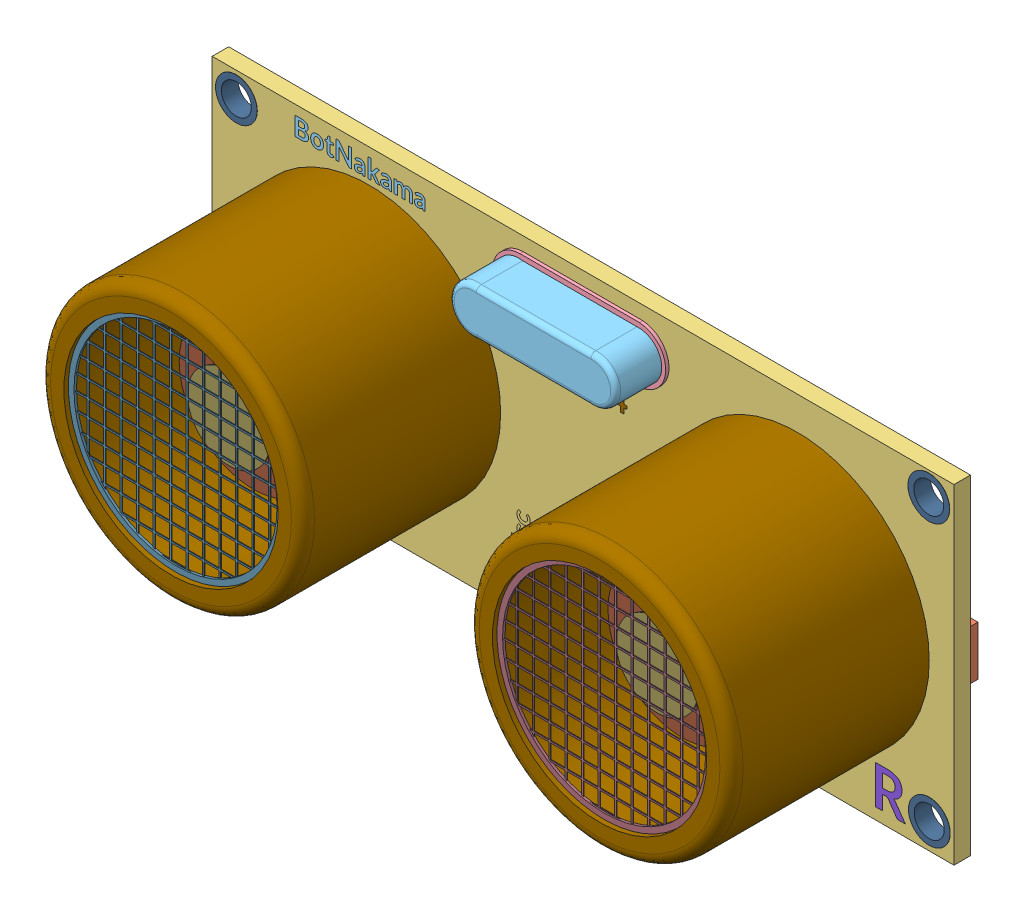
SolidWorks assembly HC-04HC-04, configuration Default. Lengths in mm.
Overall size (45 25.57 17.46).
61 component instances, 60 part files, 0 mates.
Components (placement in the parent):
- HC-04HC-04.stp-1: HC-04HC-04.stp [Default] at origin size (45 25.57 17.46)
  - HC-04Array.stp-1: HC-04Array.stp [Default] at origin size (10.16 2.54 2.54)
  - HC-04Array001.stp-1: HC-04Array001.stp [Default] at (0 0 1) size (8.32 7.52 6.46)
  - HC-04Placa.stp-1: HC-04Placa.stp [Default] at origin size (45 20 1)
  - HC-04Pad003.stp-1: HC-04Pad003.stp [Default] at (0 0 1) size (10.52 3.38 0.2)
  - HC-04Fillet.stp-1: HC-04Fillet.stp [Default] at (0 0 1) size (10.1 2.84 3)
  - HC-04Array002.stp-1: HC-04Array002.stp [Default] at origin size (9.62 2 1)
  - HC-04Array003.stp-1: HC-04Array003.stp [Default] at (0 0 1) size (28 12 0.8)
  - HC-04Fusion.stp-1: HC-04Fusion.stp [Default] at origin size (6 2 1)
  - HC-04Fillet001.stp-1: HC-04Fillet001.stp [Default] at (0 0 1) size (42 16 12)
  - HC-04Pad005.stp-1: HC-04Pad005.stp [Default] at (0 0 1) size (39.16 13 0.2)
  - HC-04Pad006.stp-1: HC-04Pad006.stp [Default] at (0 0 1) size (35.01 9.04 7)
  - HC-04Fusion001.stp-1: HC-04Fusion001.stp [Default] at (0 0 8) size (31 5 1.5)
  - HC-04Clone_of_Fusion002.stp-1: HC-04Clone_of_Fusion002.stp [Default] at (47.2 -5.5 12.6) size (13 13 0.15)
  - HC-04Clone_of_Fusion003.stp-1: HC-04Clone_of_Fusion003.stp [Default] at (21.2 -5.5 12.6) size (13 13 0.15)
  - HC-04Array005.stp-1: HC-04Array005.stp [Default] at origin size (9.62 2 1)
  - HC-04Array002002.stp-1: HC-04Array002002.stp [Default] at (-5.9 0.1 0.15) size (6.57 1.4 0.56)
  - HC-04Clone_of_Array002002.stp-1: HC-04Clone_of_Array002002.stp [Default] at (-23.9 0.1 0.15) size (6.57 1.4 0.56)
  - HC-04Array002003.stp-1: HC-04Array002003.stp [Default] at (-6.05 0 0.15) size (6.57 1.4 0.56)
  - HC-04Clone_of_Array002003.stp-1: HC-04Clone_of_Array002003.stp [Default] at (-24.05 0 0.15) size (6.57 1.4 0.56)
  - HC-04Integrados.stp-1: HC-04Integrados.stp [Default] at origin size (42.14 9 1)
  - HC-04ShapeString.stp-1: HC-04ShapeString.stp [Default] at (-3.2 -7 1.01) x (0 1 0) z (0 0 1) size (2.53 1.13 0.01)
  - HC-04ShapeString001.stp-1: HC-04ShapeString001.stp [Default] at (-0.6 -7 1.01) x (0 1 0) z (0 0 1) size (2.66 1.45 0.01)
  - HC-04ShapeString002.stp-1: HC-04ShapeString002.stp [Default] at (1.9 -7 1.01) x (0 1 0) z (0 0 1) size (3.21 1.16 0.01)
  - HC-04ShapeString003.stp-1: HC-04ShapeString003.stp [Default] at (4.5 -7 1.01) x (0 1 0) z (0 0 1) size (2.71 1.16 0.01)
  - HC-04ShapeString004.stp-1: HC-04ShapeString004.stp [Default] at (-19.5 -9.3 1.01) size (1.84 2.34 0.01)
  - HC-04ShapeString005.stp-1: HC-04ShapeString005.stp [Default] at (17.5 -9.3 1.01) size (1.82 2.34 0.01)
  - HC-04ShapeString006.stp-1: HC-04ShapeString006.stp [Default] at (-3 3.7 1.01) size (5.52 1.41 0.01)
  - HC-04Pad008.stp-1: HC-04Pad008.stp [Default] at (0 0 -0.01) size (44.56 19.6 1.02)
  - HC-04Scale004.stp-1: HC-04Scale004.stp [Default] at (-1.9 -21.5 -1.5) x (0 1 0) z (0 0 1) size (0.8 1.77 0.5)
  - HC-04Scale027.stp-1: HC-04Scale027.stp [Default] at (-1.9 -10.2323 -1.5) x (0 1 0) z (0 0 1) size (0.8 1.77 0.5)
  - HC-04Scale028.stp-1: HC-04Scale028.stp [Default] at (8.5984 -21.5 -1.5) x (0 1 0) z (0 0 1) size (0.8 1.77 0.5)
  - HC-04Scale029.stp-1: HC-04Scale029.stp [Default] at (8.5984 -19.5867 -1.5) x (0 1 0) z (0 0 1) size (0.8 1.77 0.5)
  - HC-04Scale030.stp-1: HC-04Scale030.stp [Default] at (8.5984 -17.5982 -1.5) x (0 1 0) z (0 0 1) size (0.8 1.77 0.5)
  - HC-04Scale031.stp-1: HC-04Scale031.stp [Default] at (8.5984 -15.6427 -1.5) x (0 1 0) z (0 0 1) size (0.8 1.77 0.5)
  - HC-04Scale032.stp-1: HC-04Scale032.stp [Default] at (8.5984 -11.6848 -1.5) x (0 1 0) z (0 0 1) size (0.8 1.77 0.5)
  - HC-04Scale033.stp-1: HC-04Scale033.stp [Default] at (-26.74 -2 -1.5) x (0 1 0) z (0 0 1) size (0.8 1.85 0.5)
  - HC-04Scale034.stp-1: HC-04Scale034.stp [Default] at (24.9371 -21.5 -1.5) x (0 1 0) z (0 0 1) size (0.8 1.77 0.5)
  - HC-04Scale035.stp-1: HC-04Scale035.stp [Default] at (24.9691 -19.5867 -1.5) x (0 1 0) z (0 0 1) size (0.8 1.77 0.5)
  - HC-04Scale036.stp-1: HC-04Scale036.stp [Default] at (24.9742 -17.5982 -1.5) x (0 1 0) z (0 0 1) size (0.8 1.77 0.5)
  - HC-04Scale037.stp-1: HC-04Scale037.stp [Default] at (-10.4013 -2 -1.5) x (0 1 0) z (0 0 1) size (0.8 1.85 0.5)
  - HC-04Scale038.stp-1: HC-04Scale038.stp [Default] at (-10.4013 -3.9266 -1.5) x (0 1 0) z (0 0 1) size (0.8 1.85 0.5)
  - HC-04Scale039.stp-1: HC-04Scale039.stp [Default] at (-10.4013 -0.0734 -1.5) x (0 1 0) z (0 0 1) size (0.8 1.85 0.5)
  - HC-04Scale040.stp-1: HC-04Scale040.stp [Default] at (24.9742 -9.855 -1.5) x (0 1 0) z (0 0 1) size (0.8 1.77 0.5)
  - HC-04Scale041.stp-1: HC-04Scale041.stp [Default] at (26.5673 -24.0564 -1.5) x (0 1 0) z (0 0 1) size (0.8 1.77 0.5)
  - HC-04Scale042.stp-1: HC-04Scale042.stp [Default] at (26.5673 -7.3333 -1.5) x (0 1 0) z (0 0 1) size (0.8 1.77 0.5)
  - HC-04Scale043.stp-1: HC-04Scale043.stp [Default] at (30.1435 -7.3333 -1.5) x (0 1 0) z (0 0 1) size (0.8 1.77 0.5)
  - HC-04Scale044.stp-1: HC-04Scale044.stp [Default] at (33.5459 -7.3333 -1.5) x (0 1 0) z (0 0 1) size (0.8 1.77 0.5)
  - HC-04Scale045.stp-1: HC-04Scale045.stp [Default] at (37.7181 -11.1827 -1.5) x (0 1 0) z (0 0 1) size (0.8 1.77 0.5)
  - HC-04Scale046.stp-1: HC-04Scale046.stp [Default] at (37.7181 -20.5932 -1.5) x (0 1 0) z (0 0 1) size (0.8 1.77 0.5)
  - HC-04Scale047.stp-1: HC-04Scale047.stp [Default] at (-3.9042 -12.3288 -1.5) x (0 1 0) z (0 0 1) size (0.8 1.85 0.5)
  - HC-04Scale048.stp-1: HC-04Scale048.stp [Default] at (13.5402 13.2894 -1.5) size (0.8 1.85 0.5)
  - HC-04Scale049.stp-1: HC-04Scale049.stp [Default] at (13.5402 23.7909 -1.5) size (0.8 1.85 0.5)
  - HC-04Pad009.stp-1: HC-04Pad009.stp [Default] x (1 0 0) z (0 0 -1) size (42.21 18.43 0.01)
  - HC-04ShapeString007.stp-1: HC-04ShapeString007.stp [Default] at (-3.2 -7 -0.1) x (0 1 0) z (0 0 1) size (2.53 1.13 0.01)
  - HC-04ShapeString008.stp-1: HC-04ShapeString008.stp [Default] at (-0.6 -7 -0.1) x (0 1 0) z (0 0 1) size (2.66 1.45 0.01)
  - HC-04ShapeString009.stp-1: HC-04ShapeString009.stp [Default] at (1.9 -7 -0.1) x (0 1 0) z (0 0 1) size (3.21 1.16 0.01)
  - HC-04ShapeString010.stp-1: HC-04ShapeString010.stp [Default] at (4.5 -7 -0.1) x (0 1 0) z (0 0 1) size (2.71 1.16 0.01)
  - HC-04Fusion002.stp-1: HC-04Fusion002.stp [Default] at origin size (5.7 7.57 0.56)
  - HC-04ShapeString011.stp-1: HC-04ShapeString011.stp [Default] at (-17.5 8.4 1.1) size (7.91 1.16 0.01)
  - HC-04ShapeString012.stp-1: HC-04ShapeString012.stp [Default] at (-7.5 8 -0.1) x (-1 0 0) z (0 0 -1) size (7.91 1.16 0.01)
